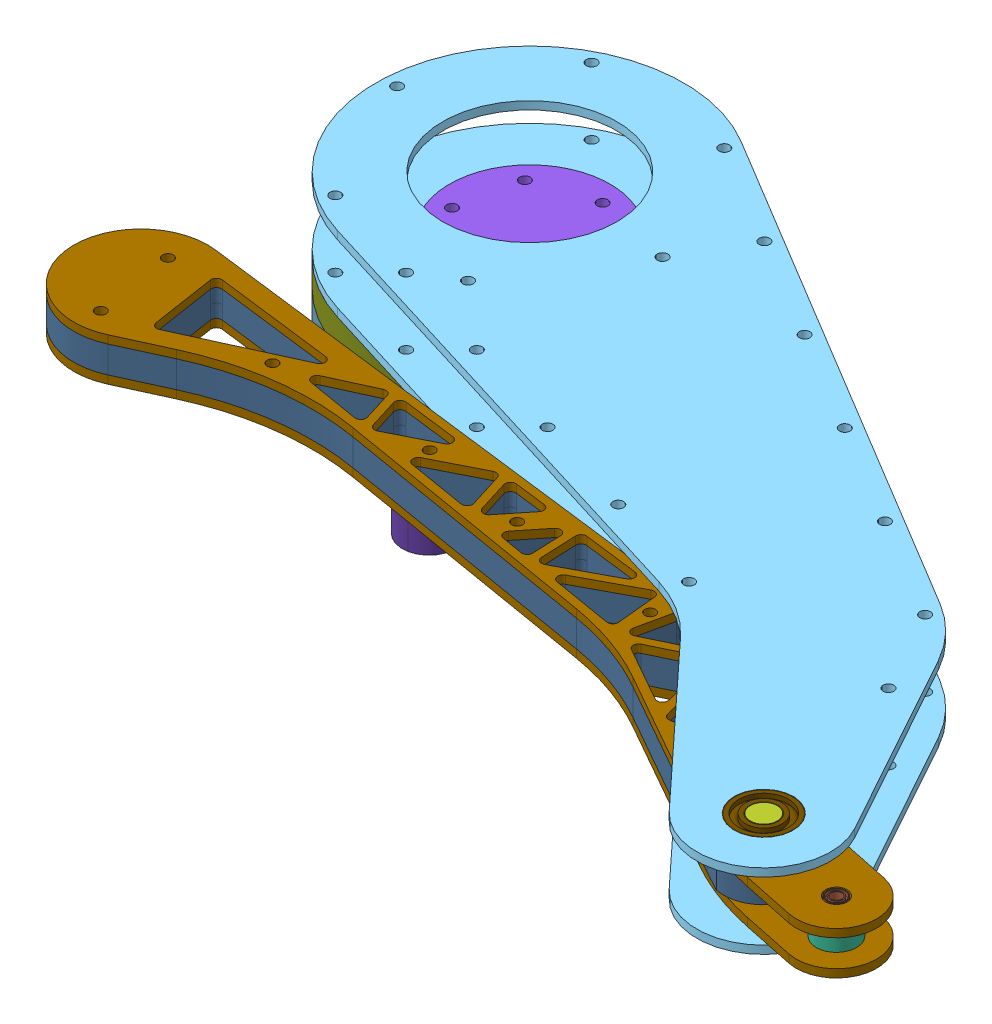
SolidWorks assembly leg, configuration Default. Lengths in mm. (continued)
Components (placement in the parent): (continued)
- Cycloidal-1: Cycloidal [Default] at (11.8169 34.4235 32.4982) x (0.945191 0 0.326517) z (-0.326517 0 0.945191) size (162.63 70.39 162.63) (continued)
  - foc-motor-controller.step-1: foc-motor-controller.step [Default] at (47.267 33.6573 89.1587) x (0.707107 0 0.707107) z (0 -1 0) size (57.23 50 8.13) (continued)
    - RTA0040B.step-1: RTA0040B.step [Default] at (12.5014 -1.6986 1.595) x (-0.707107 -0.707107 0) z (0 0 1) size (6 6 1) (continued)
      - FRAME.step-1: FRAME.step [Default] x (1 0 0) z (0 -1 0) size (6 0.2 6) (continued)
        - SOLID-2.step-1: SOLID-2.step [Default] at origin size (0.4 0.2 0.22)
        - SOLID-3.step-1: SOLID-3.step [Default] at origin size (0.4 0.2 0.22)
        - SOLID-4.step-1: SOLID-4.step [Default] at origin size (0.4 0.2 0.22)
        - SOLID-5.step-1: SOLID-5.step [Default] at origin size (0.4 0.2 0.22)
        - SOLID-6.step-1: SOLID-6.step [Default] at origin size (0.4 0.2 0.22)
        - SOLID-7.step-1: SOLID-7.step [Default] at origin size (0.4 0.2 0.22)
        - SOLID-8.step-1: SOLID-8.step [Default] at origin size (0.4 0.2 0.22)
        - SOLID-9.step-1: SOLID-9.step [Default] at origin size (0.22 0.2 0.4)
        - SOLID-10.step-1: SOLID-10.step [Default] at origin size (0.22 0.2 0.4)
        - SOLID-11.step-1: SOLID-11.step [Default] at origin size (0.22 0.2 0.4)
        - SOLID-12.step-1: SOLID-12.step [Default] at origin size (0.22 0.2 0.4)
        - SOLID-13.step-1: SOLID-13.step [Default] at origin size (0.22 0.2 0.4)
        - SOLID-14.step-1: SOLID-14.step [Default] at origin size (0.22 0.2 0.4)
        - SOLID-15.step-1: SOLID-15.step [Default] at origin size (0.22 0.2 0.4)
        - SOLID-16.step-1: SOLID-16.step [Default] at origin size (0.22 0.2 0.4)
        - SOLID-17.step-1: SOLID-17.step [Default] at origin size (4.15 0.2 4.15)
        - SOLID-18.step-1: SOLID-18.step [Default] at origin size (0.28 0.1 0.28)
        - SOLID-19.step-1: SOLID-19.step [Default] at origin size (0.28 0.1 0.28)
        - SOLID-20.step-1: SOLID-20.step [Default] at origin size (0.28 0.1 0.28)
        - SOLID-21.step-1: SOLID-21.step [Default] at origin size (0.28 0.1 0.28)
        - SOLID-22.step-1: SOLID-22.step [Default] at origin size (0.4 0.2 0.22)
        - SOLID-23.step-1: SOLID-23.step [Default] at origin size (0.4 0.2 0.22)
        - SOLID-24.step-1: SOLID-24.step [Default] at origin size (0.4 0.2 0.22)
        - SOLID-25.step-1: SOLID-25.step [Default] at origin size (0.4 0.2 0.22)
        - SOLID-26.step-1: SOLID-26.step [Default] at origin size (0.4 0.2 0.22)
        - SOLID-27.step-1: SOLID-27.step [Default] at origin size (0.4 0.2 0.22)
        - SOLID-28.step-1: SOLID-28.step [Default] at origin size (0.4 0.2 0.22)
        - SOLID-29.step-1: SOLID-29.step [Default] at origin size (0.4 0.2 0.22)
        - SOLID-30.step-1: SOLID-30.step [Default] at origin size (0.4 0.2 0.22)
        - SOLID-31.step-1: SOLID-31.step [Default] at origin size (0.4 0.2 0.22)
        - SOLID-32.step-1: SOLID-32.step [Default] at origin size (0.22 0.2 0.4)
        - SOLID-33.step-1: SOLID-33.step [Default] at origin size (0.22 0.2 0.4)
        - SOLID-34.step-1: SOLID-34.step [Default] at origin size (0.22 0.2 0.4)
        - SOLID-35.step-1: SOLID-35.step [Default] at origin size (0.22 0.2 0.4)
        - SOLID-36.step-1: SOLID-36.step [Default] at origin size (0.22 0.2 0.4)
        - SOLID-37.step-1: SOLID-37.step [Default] at origin size (0.22 0.2 0.4)
        - SOLID-38.step-1: SOLID-38.step [Default] at origin size (0.22 0.2 0.4)
        - SOLID-39.step-1: SOLID-39.step [Default] at origin size (0.22 0.2 0.4)
        - SOLID-40.step-1: SOLID-40.step [Default] at origin size (0.22 0.2 0.4)
        - SOLID-41.step-1: SOLID-41.step [Default] at origin size (0.22 0.2 0.4)
        - SOLID-42.step-1: SOLID-42.step [Default] at origin size (0.22 0.2 0.4)
        - SOLID-43.step-1: SOLID-43.step [Default] at origin size (0.22 0.2 0.4)
      - BODY.step-1: BODY.step [Default] at (0 0 0.025) x (1 0 0) z (0 -1 0) size (6 0.97 6)
    - Resonator_SMD_Murata_CSTxExxV-3Pin_3.0x1.1mm.step-1: Resonator_SMD_Murata_CSTxExxV-3Pin_3.0x1.1mm.step [Default] at (1.8 -7 1.595) x (0 1 0) z (0 0 1) size (3.2 1.35 0.9)
    - C_0603_1608Metric.step-1: C_0603_1608Metric.step [Default] at (6.2 -16.8 1.595) x (0 -1 0) z (0 0 1) size (1.6 0.8 0.8)
    - R_0603_1608Metric.step-1: R_0603_1608Metric.step [Default] at (11.8 -7.375 1.595) x (0 1 0) z (0 0 1) size (1.6 0.8 0.45)
    - R_0603_1608Metric.step-2: R_0603_1608Metric.step [Default] at (13.8 -16.8 1.595) x (0 1 0) z (0 0 1) size (1.6 0.8 0.45)
    - R_0603_1608Metric.step-3: R_0603_1608Metric.step [Default] at (18.1 -5.36 1.595) size (1.6 0.8 0.45)
    - C_0603_1608Metric.step-2: C_0603_1608Metric.step [Default] at (2.6 -0.5 1.595) x (0 -1 0) z (0 0 1) size (1.6 0.8 0.8)
    - R_0603_1608Metric.step-4: R_0603_1608Metric.step [Default] at (14.6 -11.3 1.595) x (0 1 0) z (0 0 1) size (1.6 0.8 0.45)
    - L_APV_ANR4020.step-1: L_APV_ANR4020.step [Default] at (22.3 -13.7 1.595) x (0 -1 0) z (0 0 1) size (4.02 4 2)
    - C_0603_1608Metric.step-3: C_0603_1608Metric.step [Default] at (0.3 -12.6 1.595) x (-1 0 0) z (0 0 1) size (1.6 0.8 0.8)
    - C_1206_3216Metric.step-1: C_1206_3216Metric.step [Default] at (15.7 11 1.595) x (0 1 0) z (0 0 1) size (3.2 1.6 1.6)
    - C_0603_1608Metric.step-4: C_0603_1608Metric.step [Default] at (0.3 -9.6 1.595) size (1.6 0.8 0.8)
    - R_0603_1608Metric.step-5: R_0603_1608Metric.step [Default] at (12.3 -16.8 1.595) x (0 1 0) z (0 0 1) size (1.6 0.8 0.45)
    - C_0603_1608Metric.step-5: C_0603_1608Metric.step [Default] at (-0.3 -16.6 1.595) x (0 1 0) z (0 0 1) size (1.6 0.8 0.8)
    - R_0603_1608Metric.step-6: R_0603_1608Metric.step [Default] at (10.9 4.1 1.595) size (1.6 0.8 0.45)
    - C_1206_3216Metric.step-2: C_1206_3216Metric.step [Default] at (6.3 11 1.595) x (0 1 0) z (0 0 1) size (3.2 1.6 1.6)
    - XT30PW_2_2_-M.G.B.step-1: XT30PW_2_2_-M.G.B.step [Default] at (-20.5 9.5 1.595) x (0 -1 0) z (-1 0 0) size (15.5 7.1 12.53)
    - R_0603_1608Metric.step-7: R_0603_1608Metric.step [Default] at (0.3 -11.1 1.595) size (1.6 0.8 0.45)
    - C_0603_1608Metric.step-6: C_0603_1608Metric.step [Default] at (19 -0.4 1.595) x (-0.707107 -0.707107 0) z (0 0 1) size (1.6 0.8 0.8)
    - C_1206_3216Metric.step-3: C_1206_3216Metric.step [Default] at (13.3 11 1.595) x (0 1 0) z (0 0 1) size (3.2 1.6 1.6)
    - R_0603_1608Metric.step-8: R_0603_1608Metric.step [Default] at (10.2 -7.375 1.595) x (0 -1 0) z (0 0 1) size (1.6 0.8 0.45)
    - JST_GH_SM08B-GHS-TB_1x08-1MP_P1.25mm_Horizontal.step-1: JST_GH_SM08B-GHS-TB_1x08-1MP_P1.25mm_Horizontal.step [Default] at (10 -22 1.595) size (13.25 4.95 4.25)
    - C_1206_3216Metric.step-4: C_1206_3216Metric.step [Default] at (-12.3 11 1.595) x (0 1 0) z (0 0 1) size (3.2 1.6 1.6)
    - JST_GH_SM06B-GHS-TB_1x06-1MP_P1.25mm_Horizontal.step-1: JST_GH_SM06B-GHS-TB_1x06-1MP_P1.25mm_Horizontal.step [Default] at (-4.3 -22 1.595) size (10.75 4.95 4.25)
    - C_0603_1608Metric.step-7: C_0603_1608Metric.step [Default] at (7.3 -4.5 1.595) x (-1 0 0) z (0 0 1) size (1.6 0.8 0.8)
    - R_0603_1608Metric.step-9: R_0603_1608Metric.step [Default] at (18.1 -3.86 1.595) x (-1 0 0) z (0 0 1) size (1.6 0.8 0.45)
    - C_1206_3216Metric.step-5: C_1206_3216Metric.step [Default] at (22.6794 -1.2206 1.595) x (0.707107 -0.707107 0) z (0 0 1) size (3.2 1.6 1.6)
    - R_Array_Convex_4x0402.step-1: R_Array_Convex_4x0402.step [Default] at (6.8 -2.5 1.595) size (1 2 0.35)
    - R_0603_1608Metric.step-10: R_0603_1608Metric.step [Default] at (7.7 -16.8 1.595) x (0 -1 0) z (0 0 1) size (1.6 0.8 0.45)
    - C_1206_3216Metric.step-6: C_1206_3216Metric.step [Default] at (8.7 11 1.595) x (0 1 0) z (0 0 1) size (3.2 1.6 1.6)
    - C_0603_1608Metric.step-8: C_0603_1608Metric.step [Default] at (16.1 -11.3 1.595) x (0 1 0) z (0 0 1) size (1.6 0.8 0.8)
    - SOT-23-5.step-1: SOT-23-5.step [Default] at (-3.1 -16.6 1.595) x (-1 0 0) z (0 0 1) size (2.8 2.9 1.55)
    - C_0603_1608Metric.step-9: C_0603_1608Metric.step [Default] at (17.8 -13.6 1.595) size (1.6 0.8 0.8)
    - R_0603_1608Metric.step-11: R_0603_1608Metric.step [Default] at (-11.5 -20.3875 1.595) x (0 -1 0) z (0 0 1) size (1.6 0.8 0.45)
    - C_0603_1608Metric.step-10: C_0603_1608Metric.step [Default] at (-12.4 2.3 1.595) x (0 1 0) z (0 0 1) size (1.6 0.8 0.8)
    - C_1206_3216Metric.step-7: C_1206_3216Metric.step [Default] at (18 11 1.595) x (0 1 0) z (0 0 1) size (3.2 1.6 1.6)
    - R_0603_1608Metric.step-12: R_0603_1608Metric.step [Default] at (-10.8105 -14.9971 1.595) x (-1 0 0) z (0 0 1) size (1.6 0.8 0.45)
    - C_0603_1608Metric.step-11: C_0603_1608Metric.step [Default] at (-13.8 -9.4 1.595) x (-1 0 0) z (0 0 1) size (1.6 0.8 0.8)
    - R_0603_1608Metric.step-13: R_0603_1608Metric.step [Default] at (-23.15 -14.5 1.595) x (-1 0 0) z (0 0 1) size (1.6 0.8 0.45)
    - C_0603_1608Metric.step-12: C_0603_1608Metric.step [Default] at (1.1 -0.2 1.595) x (0 1 0) z (0 0 1) size (1.6 0.8 0.8)
    - D_0805_2012Metric.step-1: D_0805_2012Metric.step [Default] at (22.9 -9.6 1.595) x (0 1 0) z (0 0 1) size (2 1.27 0.8)
    - C_0603_1608Metric.step-13: C_0603_1608Metric.step [Default] at (-7.8 3.775 1.595) x (0 -1 0) z (0 0 1) size (1.6 0.8 0.8)
    - R_0603_1608Metric.step-14: R_0603_1608Metric.step [Default] at (-6.4 -12.825 1.595) x (0 1 0) z (0 0 1) size (1.6 0.8 0.45)
    - L_0603_1608Metric.step-1: L_0603_1608Metric.step [Default] at (-10.1 3 1.595) size (1.6 0.8 0.8)
    - C_0603_1608Metric.step-14: C_0603_1608Metric.step [Default] at (17.9 0.7 1.595) x (-0.707107 -0.707107 0) z (0 0 1) size (1.6 0.8 0.8)
    - HVSSOP-10.step-1: HVSSOP-10.step [Default] at (18.6 -9.6 1.595) x (0 -1 0) z (-1 0 0) size (4.9 1.1 3)
    - C_0603_1608Metric.step-15: C_0603_1608Metric.step [Default] at (7.9 4.1 1.595) x (-1 0 0) z (0 0 1) size (1.6 0.8 0.8)
    - C_0603_1608Metric.step-16: C_0603_1608Metric.step [Default] at (21.1 -9.6 1.595) x (0 -1 0) z (0 0 1) size (1.6 0.8 0.8)
    - R_0603_1608Metric.step-15: R_0603_1608Metric.step [Default] at (-10.8105 -11.9971 1.595) x (-1 0 0) z (0 0 1) size (1.6 0.8 0.45)
    - R_0603_1608Metric.step-16: R_0603_1608Metric.step [Default] at (-18.2 -17.4 1.595) size (1.6 0.8 0.45)
    - C_1206_3216Metric.step-8: C_1206_3216Metric.step [Default] at (-3 11 1.595) x (0 1 0) z (0 0 1) size (3.2 1.6 1.6)
    - R_0603_1608Metric.step-17: R_0603_1608Metric.step [Default] at (-16.9 -20.4 1.595) x (0 -1 0) z (0 0 1) size (1.6 0.8 0.45)
    - R_0603_1608Metric.step-18: R_0603_1608Metric.step [Default] at (-13.3 -20.3875 1.595) x (0 -1 0) z (0 0 1) size (1.6 0.8 0.45)
    - R_0603_1608Metric.step-19: R_0603_1608Metric.step [Default] at (-15.1 -20.3875 1.595) x (0 -1 0) z (0 0 1) size (1.6 0.8 0.45)
    - C_0603_1608Metric.step-17: C_0603_1608Metric.step [Default] at (15.5 -14.4 1.595) x (0 -1 0) z (0 0 1) size (1.6 0.8 0.8)
    - LED_0603_1608Metric.step-1: LED_0603_1608Metric.step [Default] at (-11.5 -23.3875 1.595) x (0 1 0) z (0 0 1) size (1.6 0.8 1.1)
    - C_0805_2012Metric.step-1: C_0805_2012Metric.step [Default] at (19.95 -17 1.595) size (2 1.25 1.25)
    - D_SMB.step-1: D_SMB.step [Default] at (-16.5 11.208 1.595) x (0 -1 0) z (0 0 1) size (5.3 3.55 2.15)
    - C_1206_3216Metric.step-9: C_1206_3216Metric.step [Default] at (-5.3 11 1.595) x (0 1 0) z (0 0 1) size (3.2 1.6 1.6)
    - XT30PW_2_2_-M.G.B.step-2: XT30PW_2_2_-M.G.B.step [Default] at (-20.5 -6.5 1.595) x (0 -1 0) z (-1 0 0) size (15.5 7.1 12.53)
    - C_1206_3216Metric.step-10: C_1206_3216Metric.step [Default] at (1.7 11 1.595) x (0 1 0) z (0 0 1) size (3.2 1.6 1.6)
    - C_1206_3216Metric.step-11: C_1206_3216Metric.step [Default] at (11 11 1.595) x (0 1 0) z (0 0 1) size (3.2 1.6 1.6)
    - C_0603_1608Metric.step-18: C_0603_1608Metric.step [Default] at (-6.3 3.775 1.595) x (0 -1 0) z (0 0 1) size (1.6 0.8 0.8)
    - C_0603_1608Metric.step-19: C_0603_1608Metric.step [Default] at (16.8686 1.7314 1.595) x (0.707107 0.707107 0) z (0 0 1) size (1.6 0.8 0.8)
    - C_0603_1608Metric.step-20: C_0603_1608Metric.step [Default] at (-15.0105 -11.1 1.595) size (1.6 0.8 0.8)
    - C_1206_3216Metric.step-12: C_1206_3216Metric.step [Default] at (-7.7 11 1.595) x (0 1 0) z (0 0 1) size (3.2 1.6 1.6)
    - C_0603_1608Metric.step-21: C_0603_1608Metric.step [Default] at (-18.2 -15.8 1.595) size (1.6 0.8 0.8)
    - C_0603_1608Metric.step-22: C_0603_1608Metric.step [Default] at (-2.1 -11.3 1.595) x (0 -1 0) z (0 0 1) size (1.6 0.8 0.8)
    - C_0603_1608Metric.step-23: C_0603_1608Metric.step [Default] at (-10.8105 -13.4971 1.595) size (1.6 0.8 0.8)
    - C_1206_3216Metric.step-13: C_1206_3216Metric.step [Default] at (4 11 1.595) x (0 1 0) z (0 0 1) size (3.2 1.6 1.6)
    - R_0603_1608Metric.step-20: R_0603_1608Metric.step [Default] at (16 -17.8 1.595) x (0 1 0) z (0 0 1) size (1.6 0.8 0.45)
    - Texas_S-PVSON-N8.step-1: Texas_S-PVSON-N8.step [Default] at (-14.4105 -13.7 1.595) x (-1 0 0) z (0 0 1) size (3 2.98 0.92)
    - C_1206_3216Metric.step-14: C_1206_3216Metric.step [Default] at (21 -2.9 1.595) x (0.707107 -0.707107 0) z (0 0 1) size (3.2 1.6 1.6)
    - C_0603_1608Metric.step-24: C_0603_1608Metric.step [Default] at (-5.9 -16.6 1.595) x (0 1 0) z (0 0 1) size (1.6 0.8 0.8)
    - C_0603_1608Metric.step-25: C_0603_1608Metric.step [Default] at (-3.1 -14.1 1.595) size (1.6 0.8 0.8)
    - R_0603_1608Metric.step-21: R_0603_1608Metric.step [Default] at (7.2 -7.375 1.595) x (0 -1 0) z (0 0 1) size (1.6 0.8 0.45)
    - C_1206_3216Metric.step-15: C_1206_3216Metric.step [Default] at (-0.7 11 1.595) x (0 1 0) z (0 0 1) size (3.2 1.6 1.6)
    - LQFP-64_10x10mm_P0.5mm.step-1: LQFP-64_10x10mm_P0.5mm.step [Default] at (-7 -4.5 1.595) x (-1 0 0) z (0 0 1) size (12 12 1.5)
    - C_0805_2012Metric.step-2: C_0805_2012Metric.step [Default] at (23.35 -17 1.595) x (-1 0 0) z (0 0 1) size (2 1.25 1.25)
    - C_0603_1608Metric.step-26: C_0603_1608Metric.step [Default] at (10.8 -16.8 1.595) x (0 -1 0) z (0 0 1) size (1.6 0.8 0.8)
    - R_0603_1608Metric.step-22: R_0603_1608Metric.step [Default] at (17.5 -17.8 1.595) x (0 -1 0) z (0 0 1) size (1.6 0.8 0.45)
    - C_1206_3216Metric.step-16: C_1206_3216Metric.step [Default] at (20.3 11 1.595) x (0 1 0) z (0 0 1) size (3.2 1.6 1.6)
    - R_0603_1608Metric.step-23: R_0603_1608Metric.step [Default] at (9.2 -16.8 1.595) x (0 -1 0) z (0 0 1) size (1.6 0.8 0.45)
    - C_1206_3216Metric.step-17: C_1206_3216Metric.step [Default] at (-10 11 1.595) x (0 1 0) z (0 0 1) size (3.2 1.6 1.6)
    - R_0603_1608Metric.step-24: R_0603_1608Metric.step [Default] at (17.8 -15.2 1.595) size (1.6 0.8 0.45)
    - C_1206_3216Metric.step-18: C_1206_3216Metric.step [Default] at (19.9 2.6 1.595) x (-0.707107 0.707107 0) z (0 0 1) size (3.2 1.6 1.6)
    - C_0603_1608Metric.step-27: C_0603_1608Metric.step [Default] at (13.4 -7.375 1.595) x (0 -1 0) z (0 0 1) size (1.6 0.8 0.8)
    - R_0603_1608Metric.step-25: R_0603_1608Metric.step [Default] at (8.7 -7.375 1.595) x (0 -1 0) z (0 0 1) size (1.6 0.8 0.45)
    - PQFN-8-EP_6x5mm_P1.27mm_Generic.step-1: PQFN-8-EP_6x5mm_P1.27mm_Generic.step [Default] at (4.9 14.4 -0.085) x (0 1 0) z (0 0 -1) size (6.15 5.15 1.09)
    - C_0805_2012Metric.step-3: C_0805_2012Metric.step [Default] at (-3 8.9 -0.085) x (0 1 0) z (0 0 -1) size (2 1.25 1.25)
    - C_0603_1608Metric.step-28: C_0603_1608Metric.step [Default] at (1.5 -4.3 -0.085) x (0 1 0) z (0 0 -1) size (1.6 0.8 0.8)
    - R_2512_6332Metric.step-1: R_2512_6332Metric.step [Default] at (2.1 8.6 -0.085) x (-1 0 0) z (0 0 -1) size (6.3 3.2 0.6)
    - C_0805_2012Metric.step-4: C_0805_2012Metric.step [Default] at (18.8 8.9 -0.085) x (0 1 0) z (0 0 -1) size (2 1.25 1.25)
    - C_0805_2012Metric.step-5: C_0805_2012Metric.step [Default] at (-5.2 8.901 -0.085) x (0 1 0) z (0 0 -1) size (2 1.25 1.25)
    - PQFN-8-EP_6x5mm_P1.27mm_Generic.step-2: PQFN-8-EP_6x5mm_P1.27mm_Generic.step [Default] at (16.9 14.6 -0.085) x (0 -1 0) z (0 0 -1) size (6.15 5.15 1.09)
    - PQFN-8-EP_6x5mm_P1.27mm_Generic.step-3: PQFN-8-EP_6x5mm_P1.27mm_Generic.step [Default] at (-1.1 14.6 -0.085) x (0 -1 0) z (0 0 -1) size (6.15 5.15 1.09)
    - R_0603_1608Metric.step-26: R_0603_1608Metric.step [Default] at (8.2 8.8 -0.085) x (0 1 0) z (0 0 -1) size (1.6 0.8 0.45)
    - R_2512_6332Metric.step-2: R_2512_6332Metric.step [Default] at (-10.3 8.601 -0.085) x (1 0 0) z (0 0 -1) size (6.3 3.2 0.6)
    - TSSOP-16_4.4x5mm_P0.65mm.step-1: TSSOP-16_4.4x5mm_P0.65mm.step [Default] at (0 0 -0.085) x (-1 0 0) z (0 0 -1) size (6.4 5 1.1)
    - C_0603_1608Metric.step-29: C_0603_1608Metric.step [Default] at (0 -4.25 -0.085) x (0 1 0) z (0 0 -1) size (1.6 0.8 0.8)
    - PQFN-8-EP_6x5mm_P1.27mm_Generic.step-4: PQFN-8-EP_6x5mm_P1.27mm_Generic.step [Default] at (10.9 14.4 -0.085) x (0 1 0) z (0 0 -1) size (6.15 5.15 1.09)
    - R_2512_6332Metric.step-3: R_2512_6332Metric.step [Default] at (13.7 8.6 -0.085) x (1 0 0) z (0 0 -1) size (6.3 3.2 0.6)
    - PQFN-8-EP_6x5mm_P1.27mm_Generic.step-5: PQFN-8-EP_6x5mm_P1.27mm_Generic.step [Default] at (-13.1 14.401 -0.085) x (0 1 0) z (0 0 -1) size (6.15 5.15 1.09)
    - C_0603_1608Metric.step-30: C_0603_1608Metric.step [Default] at (-1.5 -4.3 -0.085) x (0 -1 0) z (0 0 -1) size (1.6 0.8 0.8)
    - PQFN-8-EP_6x5mm_P1.27mm_Generic.step-6: PQFN-8-EP_6x5mm_P1.27mm_Generic.step [Default] at (-7.1 14.601 -0.085) x (0 -1 0) z (0 0 -1) size (6.15 5.15 1.09)
    - foc-motor-controller_PCB.step-1: foc-motor-controller_PCB.step [Default] at origin size (50 50 1.51)
  - hex nut style 1 gradeab_iso-1: hex nut style 1 gradeab_iso [ISO - 4032 - M3 - W - N] at (47.267 33.6573 58.7531) x (1 0 0) z (0 -1 0) size (5.5 6.35 2.4)
- leg_upper-1: leg_upper [Default] at (27.3814 131.6808 132.2037) x (0.837613 0 0.546264) z (-0.546264 0 0.837613) size (382.5 3 122.85)
- link_rod-1: link_rod [Default] at (61.6493 140.6808 139.3248) x (0.837613 0 0.546264) z (-0.546264 0 0.837613) size (315 10 15)
- m10-1: m10 [Default] at (278.6654 145.6808 296.0827) x (1 0 0.000222) z (-0.000222 0 1) size (10 28 10)
- Link_Rod_2-1: Link_Rod_2 [Default] at (27.3814 135.6808 132.2037) x (-0.203462 0 0.979083) z (-0.979083 0 -0.203462) size (60 5 70)
- leg_upper-2: leg_upper [Default] at (27.3814 156.6808 132.2037) x (0.837613 0 0.546264) z (-0.546264 0 0.837613) size (382.5 3 122.85)
- Leg_Lower_out-1: Leg_Lower_out [Default] at (278.6654 137.6808 296.0827) x (0.979083 0 0.203462) z (-0.203462 0 0.979083) size (375 3 65.43)
- Leg_Lower_in-1: Leg_Lower_in [Default] at (278.6654 145.6808 296.0827) x (0.979083 0 0.203462) z (-0.203462 0 0.979083) size (339.42 10 65.43)
- Leg_Lower_out-2: Leg_Lower_out [Default] at (278.6654 150.6808 296.0827) x (0.979083 0 0.203462) z (-0.203462 0 0.979083) size (375 3 65.43)
- angular contact ball bearing_68_iso-1: angular contact ball bearing_68_iso [ISO 15 ABB - 374 - 14,SI,NC,14_68] at (312.9333 139.1808 303.2039) x (0 -1 0) z (0 0 1) size (3 7 7)
- angular contact ball bearing_68_iso-2: angular contact ball bearing_68_iso [ISO 15 ABB - 374 - 14,SI,NC,14_68] at (312.9333 152.1808 303.2039) x (0 -1 0) z (0.00016 0 1) size (3 7 7)
- radial ball bearing_68_iso-2: radial ball bearing_68_iso [ISO 15 RBB - 1910 - 10,SI,NC,10_68] at (278.6654 156.6808 296.0827) x (0 1 0) z (0 0 1) size (6 22 22)
- radial ball bearing_68_iso-4: radial ball bearing_68_iso [ISO 15 RBB - 1910 - 10,SI,NC,10_68] at (278.6654 134.6808 296.0827) x (0 1 0) z (0 0 1) size (6 22 22)
Mates (geometry in assembly coordinates):
- Concentric1: concentric anti-aligned: cylinder of Cycloidal-1/Cover-1 through (27.3814 131.6808 132.2037) axis (0 -1 0) radius 57.5; cylinder of Leg_Upper-1 through (27.3814 134.6808 132.2037) axis (0 1 0) radius 32.5
- Coincident6: coincident anti-aligned: plane of Cycloidal-1/Cover-1 through (27.3814 131.6808 132.2037) normal (0 1 0); plane of Leg_Upper-1 through (27.3814 131.6808 132.2037) normal (0 -1 0)
- Coincident7: coincident aligned: plane of Leg_Upper-1 through (27.3814 131.6808 132.2037) normal (0 -1 0); plane of m10-1 through (278.6654 131.6808 296.0827) normal (0 -1 0)
- Coincident8: coincident aligned: circle of Link_Rod-1; plane of Link_Rod_2-1 through (27.3814 140.6808 132.2037) normal (0 1 0)
- Concentric6: concentric aligned: cylinder of Link_Rod-1 through (61.6493 150.6808 139.3248) axis (0 -1 0) radius 2; cylinder of Link_Rod_2-1 through (61.6493 140.6808 139.3248) axis (0 -1 0) radius 2.5
- Concentric8: concentric aligned: cylinder of Leg_Upper-1 through (27.3814 134.6808 132.2037) axis (0 -1 0) radius 32.5; cylinder of Link_Rod_2-1 through (27.3814 140.6808 132.2037) axis (0 -1 0) radius 30
- Concentric9: concentric aligned: cylinder of Link_Rod_2-1 through (27.3814 140.6808 132.2037) axis (0 -1 0) radius 30; cylinder of Leg_Upper-2 through (27.3814 159.6808 132.2037) axis (0 -1 0) radius 32.5
- Coincident12: coincident aligned: plane of m10-1 through (278.6654 159.6808 296.0827) normal (0 1 0); plane of Leg_Upper-2 through (27.3814 159.6808 132.2037) normal (0 1 0)
- Concentric10: concentric anti-aligned: cylinder of m10-1 through (278.6654 131.6808 296.0827) axis (0 1 0) radius 5; cylinder of Leg_Upper-2 through (278.6654 159.6808 296.0827) axis (0 -1 0) radius 11
- Concentric11: concentric anti-aligned: cylinder of m10-1 through (278.6654 131.6808 296.0827) axis (0 1 0) radius 5; cylinder of Leg_Lower_out-1 through (278.6654 140.6808 296.0827) axis (0 -1 0) radius 5
- Concentric12: concentric aligned: cylinder of Link_Rod-1 through (312.9333 150.6808 303.2039) axis (0 -1 0) radius 2; cylinder of Leg_Lower_out-1 through (312.9333 140.6808 303.2039) axis (0 -1 0) radius 4
- Concentric13: concentric anti-aligned: cylinder of Leg_Upper-1 through (278.6654 134.6808 296.0827) axis (0 -1 0) radius 11; cylinder of m10-1 through (278.6654 131.6808 296.0827) axis (0 1 0) radius 5
- Coincident16: coincident aligned: plane of m10-1 through (278.6654 145.6808 296.0827) normal (0 1 0); plane of Leg_Lower_in-1 through (278.6654 145.6808 296.0827) normal (0 1 0)
- Concentric15: concentric aligned: cylinder of m10-1 through (278.6654 131.6808 296.0827) axis (0 1 0) radius 5; cylinder of Leg_Lower_in-1 through (278.6654 140.6808 296.0827) axis (0 1 0) radius 5
- Coincident17: coincident aligned: plane of Leg_Lower_out-1 through (0.8499 137.6808 247.5623) normal (-0.415816 0 -0.909449); plane of Leg_Lower_in-1 through (0.8499 145.6808 247.5623) normal (-0.415816 0 -0.909449)
- Coincident18: coincident anti-aligned: plane of Leg_Lower_out-1 through (278.6654 140.6808 296.0827) normal (0 1 0); plane of Leg_Lower_in-1 through (278.6654 140.6808 296.0827) normal (0 -1 0)
- Coincident19: coincident aligned: cylinder of m10-1 through (278.6654 131.6808 296.0827) axis (0 1 0) radius 5; circle of Leg_Lower_out-2
- Coincident20: coincident anti-aligned: plane of Leg_Lower_in-1 through (278.6654 150.6808 296.0827) normal (0 1 0); plane of Leg_Lower_out-2 through (278.6654 150.6808 296.0827) normal (0 -1 0)
- Coincident21: coincident aligned: plane of Leg_Lower_in-1 through (0.8499 145.6808 247.5623) normal (-0.415816 0 -0.909449); plane of Leg_Lower_out-2 through (0.8499 150.6808 247.5623) normal (-0.415816 0 -0.909449)
- Concentric16: concentric anti-aligned: cylinder of Leg_Lower_out-1 through (312.9333 140.6808 303.2039) axis (0 -1 0) radius 4; circle of angular contact ball bearing_68_iso-1
- Coincident23: coincident aligned: plane of Leg_Lower_out-1 through (278.6654 137.6808 296.0827) normal (0 -1 0); plane of angular contact ball bearing_68_iso-1 through (316.3533 137.6808 303.2039) normal (0 -1 0)
- Concentric171: concentric aligned: cylinder of Leg_Lower_out-2 through (312.9333 153.6808 303.2039) axis (0 -1 0) radius 4; cylinder of angular contact ball bearing_68_iso-2 through (312.9333 172.8183 303.2039) axis (0 -1 0) radius 2
- Coincident24: coincident anti-aligned: plane of Leg_Lower_out-2 through (278.6654 153.6808 296.0827) normal (0 1 0); circle of angular contact ball bearing_68_iso-2
- Coincident25: coincident anti-aligned: plane of Link_Rod-1 through (312.9333 150.6808 303.2039) normal (0 1 0); plane of Leg_Lower_out-2 through (278.6654 150.6808 296.0827) normal (0 -1 0)
- Concentric18: concentric anti-aligned: cylinder of Leg_Upper-2 through (278.6654 159.6808 296.0827) axis (0 -1 0) radius 11; cylinder of radial ball bearing_68_iso-2 through (278.6654 136.0433 296.0827) axis (0 1 0) radius 5
- Coincident26: coincident aligned: plane of Leg_Upper-2 through (27.3814 159.6808 132.2037) normal (0 1 0); plane of radial ball bearing_68_iso-2 through (267.9654 159.6808 296.0827) normal (0 1 0)
- Concentric19: concentric anti-aligned: cylinder of Leg_Upper-1 through (278.6654 134.6808 296.0827) axis (0 -1 0) radius 11; cylinder of radial ball bearing_68_iso-4 through (278.6654 114.0433 296.0827) axis (0 1 0) radius 11
- Coincident27: coincident aligned: plane of Leg_Upper-1 through (27.3814 131.6808 132.2037) normal (0 -1 0); plane of radial ball bearing_68_iso-4 through (271.8654 131.6808 296.0827) normal (0 -1 0)
